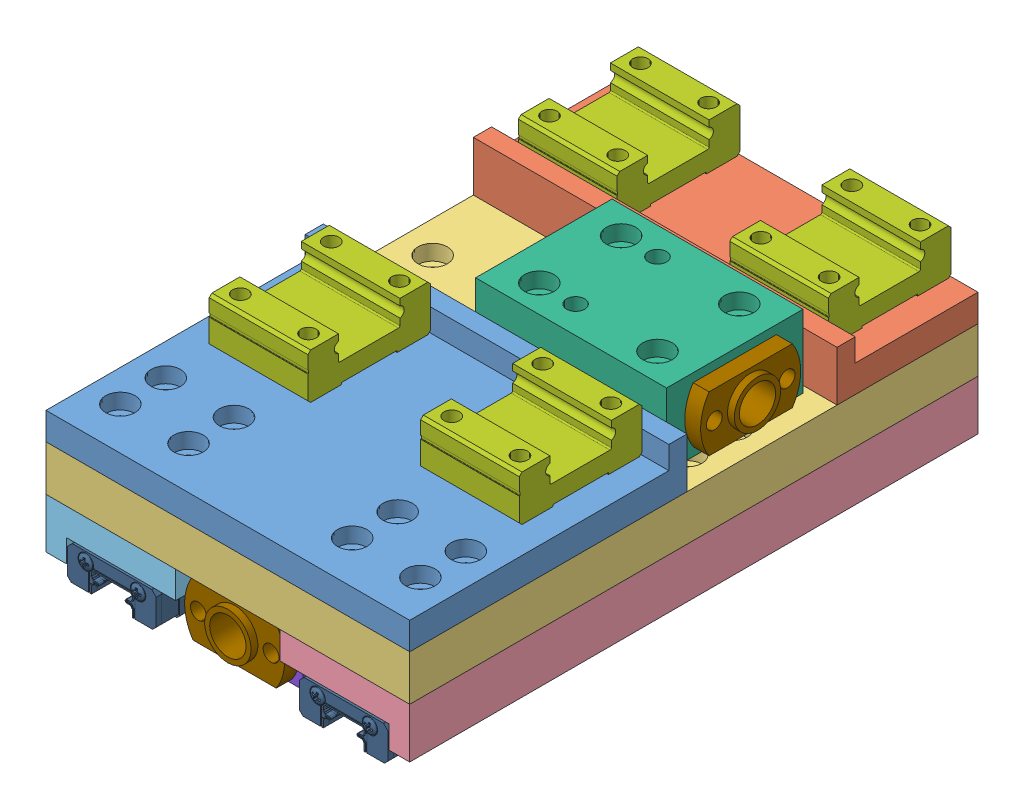
SolidWorks assembly Eje_Y, configuration Predeterminado. Lengths in mm.
Overall size (81.36 40 125.46).
19 component instances, 11 part files, 52 mates.
Components (placement in the parent):
- Copia de Alza_patines_A^Eje_Y-1: Copia de Alza_patines_A^Eje_Y [Predeterminado] at (-20.6004 -37.0232 -21.5043) x (-1 0 0) z (0 1 0) size (80 61 11) (virtual)
- Copia de Alza_patines_B^Eje_Y-1: Copia de Alza_patines_B^Eje_Y [Predeterminado] at (-20.6004 -37.0232 -85.5043) x (-1 0 0) z (0 1 0) size (80 31 11) (virtual)
- Copia de  Placa_80mm^Eje_Y-1: Copia de  Placa_80mm^Eje_Y [Predeterminado] at (-100.6004 -37.0232 -85.5043) x (1 0 0) z (0 -1 0) size (80 125 10) (virtual)
- Copia de Alza_eje_Z_A^Eje_Y-1: Copia de Alza_eje_Z_A^Eje_Y [Predeterminado] at (-49.1004 -47.0232 -85.5043) x (1 0 0) z (0 -1 0) size (28.5 125 11) (virtual)
- Copia de Alza_eje_Z_B^Eje_Y-1: Copia de Alza_eje_Z_B^Eje_Y [Predeterminado] at (-100.6004 -47.0232 -85.5043) x (1 0 0) z (0 -1 0) size (28.5 125 11) (virtual)
- Copia de Alojamiento_tuerca_Y^Eje_Y-1: Copia de Alojamiento_tuerca_Y^Eje_Y [Predeterminado] at (-26.6004 -21.0232 -23.0043) x (-1 0 0) z (0 -1 0) size (42 30 16) (virtual)
- Copia de MGN12C^Eje_Y-1: Copia de MGN12C^Eje_Y [Default] at (-28.259 -21.0071 -68.6923) x (0 0 -1) z (-1 0 0) size (27 10 34.86) (virtual)
- Copia de MGN12C^Eje_Y-2: Copia de MGN12C^Eje_Y [Default] at (-74.759 -21.0071 -68.6923) x (0 0 -1) z (-1 0 0) size (27 10 34.86) (virtual)
- Copia de MGN12C^Eje_Y-3: Copia de MGN12C^Eje_Y [Default] at (-74.759 -21.0071 -0.6923) x (0 0 -1) z (-1 0 0) size (27 10 34.86) (virtual)
- Copia de MGN12C^Eje_Y-4: Copia de MGN12C^Eje_Y [Default] at (-28.259 -21.0071 -0.6923) x (0 0 -1) z (-1 0 0) size (27 10 34.86) (virtual)
- Copia de Alojamiento_tuerca_ejeZ^Eje_Y-1: Copia de Alojamiento_tuerca_ejeZ^Eje_Y [Predeterminado] at (-49.1004 -47.0232 4.4957) x (-1 0 0) z (0 0 1) size (23 14 30) (virtual)
- Copia de eje_Y_LeadScrew_Nut_8mm_x_2mmPitch^Eje_Y-1: Copia de eje_Y_LeadScrew_Nut_8mm_x_2mmPitch^Eje_Y [Default] at (-23.1004 -29.0232 -38.0043) x (0 -1 0) z (1 0 0) size (12.2 22 15) (virtual)
- Copia de MGN9C^Eje_Y-1: Copia de MGN9C^Eje_Y [Default] at (-37.8808 -57.6723 26.1718) x (-1 0 0) z (0 0 -1) size (20 8 29.63) (virtual)
- Copia de MGN9C^Eje_Y-2: Copia de MGN9C^Eje_Y [Default] at (-83.3201 -57.6723 24.1196) size (20 8 29.63) (virtual)
- Copia de MGN9C^Eje_Y-3: Copia de MGN9C^Eje_Y [Default] at (-83.3201 -57.6723 -34.5804) size (20 8 29.63) (virtual)
- Copia de MGN9C^Eje_Y-4: Copia de MGN9C^Eje_Y [Default] at (-37.8808 -57.6723 -32.5282) x (-1 0 0) z (0 0 -1) size (20 8 29.63) (virtual)
- Copia de eje_Y_LeadScrew_Nut_8mm_x_2mmPitch^Eje_Y-2: Copia de eje_Y_LeadScrew_Nut_8mm_x_2mmPitch^Eje_Y [Default] at (-60.6004 -54.0232 37.9957) x (0 -1 0) z (0 0 1) size (12.2 22 15) (virtual)
- esquina^Eje_Y-1: esquina^Eje_Y [Predeterminado] at (-72.1004 -47.0232 4.4957) x (0 0 -1) z (0 -1 0) size (6 6 6) (virtual)
- esquina^Eje_Y-2: esquina^Eje_Y [Predeterminado] at (-49.1004 -47.0232 4.4957) x (-1 0 0) z (0 -1 0) size (6 6 6) (virtual)
Mates (geometry in assembly coordinates):
- Distancia23: distance = 68 mm: moEndPointRef_w of Copia de MGN12C^Eje_Y-1; moEndPointRef_w of Copia de MGN12C^Eje_Y-4
- Distancia22: distance = 6 mm aligned: plane of Copia de Alojamiento_tuerca_Y^Eje_Y-1 through (-26.6004 -37.0232 -23.0043) normal (1 0 0); plane of Copia de  Placa_80mm^Eje_Y-1 through (-20.6004 -47.0232 -85.5043) normal (1 0 0)
- Coincidente267: coincident anti-aligned: plane of Copia de Alojamiento_tuerca_Y^Eje_Y-1 through (-26.6004 -37.0232 -23.0043) normal (0 -1 0); plane of Copia de  Placa_80mm^Eje_Y-1 through (-100.6004 -37.0232 -85.5043) normal (0 1 0)
- Concéntrica1: concentric anti-aligned: cylinder of Copia de Alojamiento_tuerca_Y^Eje_Y-1 through (-26.6004 -29.0232 -38.0043) axis (-1 0 0) radius 5.1; cylinder of Copia de eje_Y_LeadScrew_Nut_8mm_x_2mmPitch^Eje_Y-1 through (-36.6004 -29.0232 -38.0043) axis (1 0 0) radius 5.1
- Coincidente278: coincident anti-aligned: plane of Copia de Alojamiento_tuerca_Y^Eje_Y-1 through (-26.6004 -37.0232 -23.0043) normal (1 0 0); plane of Copia de eje_Y_LeadScrew_Nut_8mm_x_2mmPitch^Eje_Y-1 through (-26.6004 -29.0232 -38.0043) normal (-1 0 0)
- Paralelo2: parallel aligned: plane of Copia de Alojamiento_tuerca_Y^Eje_Y-1 through (-26.6004 -21.0232 -23.0043) normal (0 1 0); plane of Copia de eje_Y_LeadScrew_Nut_8mm_x_2mmPitch^Eje_Y-1 through (-26.6004 -22.9232 -28.8506) normal (0 1 0)
- Coincidente285: coincident anti-aligned: plane of Copia de Alza_patines_A^Eje_Y-1 through (-20.6004 -37.0232 -21.5043) normal (0 -1 0); plane of Copia de  Placa_80mm^Eje_Y-1 through (-100.6004 -37.0232 -85.5043) normal (0 1 0)
- Coincidente286: coincident aligned: plane of Copia de Alza_patines_A^Eje_Y-1 through (-20.6004 -31.0232 -21.5043) normal (1 0 0); plane of Copia de  Placa_80mm^Eje_Y-1 through (-20.6004 -47.0232 -85.5043) normal (1 0 0)
- Coincidente287: coincident anti-aligned: plane of Copia de Alza_patines_B^Eje_Y-1 through (-20.6004 -37.0232 -85.5043) normal (0 -1 0); plane of Copia de  Placa_80mm^Eje_Y-1 through (-100.6004 -37.0232 -85.5043) normal (0 1 0)
- Coincidente288: coincident aligned: plane of Copia de Alza_patines_B^Eje_Y-1 through (-20.6004 -31.0232 -54.5043) normal (1 0 0); plane of Copia de  Placa_80mm^Eje_Y-1 through (-20.6004 -47.0232 -85.5043) normal (1 0 0)
- Coincidente289: coincident aligned: plane of Copia de Alza_patines_B^Eje_Y-1 through (-100.6004 -31.0232 -85.5043) normal (0 0 -1); plane of Copia de  Placa_80mm^Eje_Y-1 through (-100.6004 -47.0232 -85.5043) normal (0 0 -1)
- Coincidente290: coincident anti-aligned: plane of Copia de Alza_patines_A^Eje_Y-1 through (-20.6004 -26.0232 -17.5043) normal (0 0 1); plane of Copia de MGN12C^Eje_Y-4 through (-48.2004 -21.0232 -17.5043) normal (0 0 -1)
- Coincidente291: coincident anti-aligned: plane of Copia de Alza_patines_A^Eje_Y-1 through (-20.6004 -31.0232 -21.5043) normal (0 1 0); plane of Copia de MGN12C^Eje_Y-4 through (-48.2004 -31.0232 -17.5043) normal (0 -1 0)
- Coincidente292: coincident anti-aligned: plane of Copia de Alza_patines_B^Eje_Y-1 through (-20.6004 -31.0232 -85.5043) normal (0 1 0); plane of Copia de MGN12C^Eje_Y-1 through (-48.2004 -31.0232 -85.5043) normal (0 -1 0)
- Coincidente293: coincident anti-aligned: plane of Copia de Alza_patines_B^Eje_Y-1 through (-20.6004 -26.0232 -58.5043) normal (0 0 -1); plane of Copia de MGN12C^Eje_Y-1 through (-48.2004 -21.0232 -58.5043) normal (0 0 1)
- Coincidente294: coincident aligned: plane of Copia de Alza_patines_B^Eje_Y-1 through (-20.6004 -31.0232 -54.5043) normal (1 0 0); plane of Copia de MGN12C^Eje_Y-1 through (-20.6004 -30.7732 -85.2006) normal (1 0 0)
- Coincidente295: coincident aligned: plane of Copia de Alza_patines_A^Eje_Y-1 through (-20.6004 -31.0232 -21.5043) normal (1 0 0); plane of Copia de MGN12C^Eje_Y-4 through (-20.6004 -30.7732 -17.2006) normal (1 0 0)
- Coincidente296: coincident anti-aligned: plane of Copia de Alza_patines_B^Eje_Y-1 through (-20.6004 -26.0232 -58.5043) normal (0 0 -1); plane of Copia de MGN12C^Eje_Y-2 through (-94.7004 -21.0232 -58.5043) normal (0 0 1)
- Coincidente297: coincident aligned: plane of Copia de Alza_patines_B^Eje_Y-1 through (-100.6004 -31.0232 -54.5043) normal (-1 0 0); plane of Copia de MGN12C^Eje_Y-2 through (-100.6004 -30.7732 -58.7543) normal (-1 0 0)
- Coincidente298: coincident anti-aligned: plane of Copia de Alza_patines_B^Eje_Y-1 through (-20.6004 -31.0232 -85.5043) normal (0 1 0); plane of Copia de MGN12C^Eje_Y-2 through (-94.7004 -31.0232 -85.5043) normal (0 -1 0)
- Coincidente299: coincident anti-aligned: plane of Copia de Alza_patines_A^Eje_Y-1 through (-20.6004 -31.0232 -21.5043) normal (0 1 0); plane of Copia de MGN12C^Eje_Y-3 through (-94.7004 -31.0232 -17.5043) normal (0 -1 0)
- Coincidente300: coincident anti-aligned: plane of Copia de Alza_patines_A^Eje_Y-1 through (-20.6004 -26.0232 -17.5043) normal (0 0 1); plane of Copia de MGN12C^Eje_Y-3 through (-94.7004 -21.0232 -17.5043) normal (0 0 -1)
- Coincidente301: coincident aligned: plane of Copia de Alza_patines_A^Eje_Y-1 through (-100.6004 -31.0232 -21.5043) normal (-1 0 0); plane of Copia de MGN12C^Eje_Y-3 through (-100.6004 -30.7732 9.2457) normal (-1 0 0)
- Distancia35: distance = 1.5 mm anti-aligned: plane of Copia de Alza_patines_B^Eje_Y-1 through (-100.6004 -31.0232 -54.5043) normal (0 0 1); plane of Copia de Alojamiento_tuerca_Y^Eje_Y-1 through (-26.6004 -37.0232 -53.0043) normal (0 0 -1)
- Coincidente303: coincident aligned: circle of Copia de Alojamiento_tuerca_ejeZ^Eje_Y-1; circle of Copia de eje_Y_LeadScrew_Nut_8mm_x_2mmPitch^Eje_Y-2
- Coincidente304: coincident anti-aligned: plane of Copia de  Placa_80mm^Eje_Y-1 through (-100.6004 -47.0232 -85.5043) normal (0 -1 0); plane of Copia de Alojamiento_tuerca_ejeZ^Eje_Y-1 through (-49.1004 -47.0232 34.4957) normal (0 1 0)
- Distancia36: distance = 5 mm aligned: plane of Copia de  Placa_80mm^Eje_Y-1 through (-100.6004 -47.0232 39.4957) normal (0 0 1); plane of Copia de Alojamiento_tuerca_ejeZ^Eje_Y-1 through (-49.1004 -47.0232 34.4957) normal (0 0 1)
- Paralelo3: parallel aligned: plane of Copia de Alojamiento_tuerca_ejeZ^Eje_Y-1 through (-49.1004 -61.0232 34.4957) normal (0 -1 0); plane of Copia de eje_Y_LeadScrew_Nut_8mm_x_2mmPitch^Eje_Y-2 through (-69.7541 -60.1232 34.4957) normal (0 -1 0)
- Coincidente305: coincident anti-aligned: plane of Copia de  Placa_80mm^Eje_Y-1 through (-100.6004 -47.0232 -85.5043) normal (0 -1 0); plane of Copia de Alza_eje_Z_B^Eje_Y-1 through (-100.6004 -47.0232 -85.5043) normal (0 1 0)
- Coincidente306: coincident aligned: plane of Copia de  Placa_80mm^Eje_Y-1 through (-100.6004 -47.0232 39.4957) normal (0 0 1); plane of Copia de Alza_eje_Z_B^Eje_Y-1 through (-100.6004 -53.0232 39.4957) normal (0 0 1)
- Coincidente307: coincident aligned: plane of Copia de  Placa_80mm^Eje_Y-1 through (-100.6004 -47.0232 -85.5043) normal (-1 0 0); plane of Copia de Alza_eje_Z_B^Eje_Y-1 through (-100.6004 -53.0232 -85.5043) normal (-1 0 0)
- Coincidente309: coincident anti-aligned: plane of Copia de Alza_eje_Z_B^Eje_Y-1 through (-96.1004 -58.0232 -85.5043) normal (1 0 0); plane of Copia de MGN9C^Eje_Y-2 through (-96.1004 -61.0232 34.5957) normal (-1 0 0)
- Coincidente310: coincident aligned: plane of Copia de Alza_eje_Z_B^Eje_Y-1 through (-100.6004 -53.0232 39.4957) normal (0 0 1); plane of Copia de MGN9C^Eje_Y-2 through (-95.8504 -53.5232 39.4957) normal (0 0 1)
- Coincidente311: coincident anti-aligned: plane of Copia de Alza_eje_Z_B^Eje_Y-1 through (-100.6004 -53.0232 -85.5043) normal (0 -1 0); plane of Copia de MGN9C^Eje_Y-2 through (-76.1004 -53.0232 34.5957) normal (0 1 0)
- Distancia37: distance = 30 mm anti-aligned: plane of Copia de MGN9C^Eje_Y-3 through (-95.8504 -53.5232 -19.2043) normal (0 0 1); plane of Copia de MGN9C^Eje_Y-2 through (-76.3504 -53.5232 10.7957) normal (0 0 -1)
- Coincidente313: coincident anti-aligned: plane of Copia de Alza_eje_Z_B^Eje_Y-1 through (-100.6004 -53.0232 -85.5043) normal (0 -1 0); plane of Copia de MGN9C^Eje_Y-3 through (-76.1004 -53.0232 -24.1043) normal (0 1 0)
- Coincidente314: coincident anti-aligned: plane of Copia de Alza_eje_Z_B^Eje_Y-1 through (-96.1004 -58.0232 -85.5043) normal (1 0 0); plane of Copia de MGN9C^Eje_Y-3 through (-96.1004 -61.0232 -24.1043) normal (-1 0 0)
- Coincidente315: coincident aligned: plane of Copia de  Placa_80mm^Eje_Y-1 through (-100.6004 -47.0232 39.4957) normal (0 0 1); plane of Copia de Alza_eje_Z_A^Eje_Y-1 through (-49.1004 -53.0232 39.4957) normal (0 0 1)
- Coincidente316: coincident anti-aligned: plane of Copia de  Placa_80mm^Eje_Y-1 through (-100.6004 -47.0232 -85.5043) normal (0 -1 0); plane of Copia de Alza_eje_Z_A^Eje_Y-1 through (-49.1004 -47.0232 -85.5043) normal (0 1 0)
- Coincidente317: coincident aligned: plane of Copia de  Placa_80mm^Eje_Y-1 through (-20.6004 -47.0232 -85.5043) normal (1 0 0); plane of Copia de Alza_eje_Z_A^Eje_Y-1 through (-20.6004 -53.0232 -85.5043) normal (1 0 0)
- Coincidente318: coincident aligned: plane of Copia de Alza_eje_Z_A^Eje_Y-1 through (-49.1004 -53.0232 39.4957) normal (0 0 1); plane of Copia de MGN9C^Eje_Y-1 through (-44.8504 -53.5232 39.4957) normal (0 0 1)
- Coincidente319: coincident anti-aligned: plane of Copia de Alza_eje_Z_A^Eje_Y-1 through (-25.1004 -58.0232 -85.5043) normal (-1 0 0); plane of Copia de MGN9C^Eje_Y-1 through (-25.1004 -61.0232 15.6957) normal (1 0 0)
- Coincidente320: coincident anti-aligned: plane of Copia de Alza_eje_Z_A^Eje_Y-1 through (-49.1004 -53.0232 -85.5043) normal (0 -1 0); plane of Copia de MGN9C^Eje_Y-1 through (-45.1004 -53.0232 15.6957) normal (0 1 0)
- Coincidente321: coincident anti-aligned: plane of Copia de Alza_eje_Z_A^Eje_Y-1 through (-25.1004 -58.0232 -85.5043) normal (-1 0 0); plane of Copia de MGN9C^Eje_Y-4 through (-25.1004 -61.0232 -43.0043) normal (1 0 0)
- Coincidente322: coincident anti-aligned: plane of Copia de Alza_eje_Z_A^Eje_Y-1 through (-49.1004 -53.0232 -85.5043) normal (0 -1 0); plane of Copia de MGN9C^Eje_Y-4 through (-45.1004 -53.0232 -43.0043) normal (0 1 0)
- Distancia38: distance = 30 mm anti-aligned: plane of Copia de MGN9C^Eje_Y-4 through (-44.8504 -53.5232 -19.2043) normal (0 0 1); plane of Copia de MGN9C^Eje_Y-1 through (-25.3504 -53.5232 10.7957) normal (0 0 -1)
- Coincidente324: coincident anti-aligned: plane of Copia de  Placa_80mm^Eje_Y-1 through (-100.6004 -47.0232 -85.5043) normal (0 -1 0); plane of esquina^Eje_Y-1 through (-66.1004 -47.0232 -1.5043) normal (0 1 0)
- Coincidente325: coincident anti-aligned: plane of Copia de Alza_eje_Z_B^Eje_Y-1 through (-72.1004 -53.0232 -85.5043) normal (1 0 0); plane of esquina^Eje_Y-1 through (-72.1004 -53.0232 4.4957) normal (-1 0 0)
- Coincidente326: coincident anti-aligned: plane of Copia de Alojamiento_tuerca_ejeZ^Eje_Y-1 through (-49.1004 -47.0232 4.4957) normal (0 0 -1); plane of esquina^Eje_Y-1 through (-72.1004 -53.0232 4.4957) normal (0 0 1)
- Coincidente327: coincident anti-aligned: plane of Copia de  Placa_80mm^Eje_Y-1 through (-100.6004 -47.0232 -85.5043) normal (0 -1 0); plane of esquina^Eje_Y-2 through (-55.1004 -47.0232 -1.5043) normal (0 1 0)
- Coincidente328: coincident anti-aligned: plane of Copia de Alojamiento_tuerca_ejeZ^Eje_Y-1 through (-49.1004 -47.0232 4.4957) normal (0 0 -1); plane of esquina^Eje_Y-2 through (-49.1004 -53.0232 4.4957) normal (0 0 1)
- Coincidente329: coincident anti-aligned: plane of Copia de Alza_eje_Z_A^Eje_Y-1 through (-49.1004 -53.0232 -85.5043) normal (-1 0 0); plane of esquina^Eje_Y-2 through (-49.1004 -53.0232 4.4957) normal (1 0 0)
